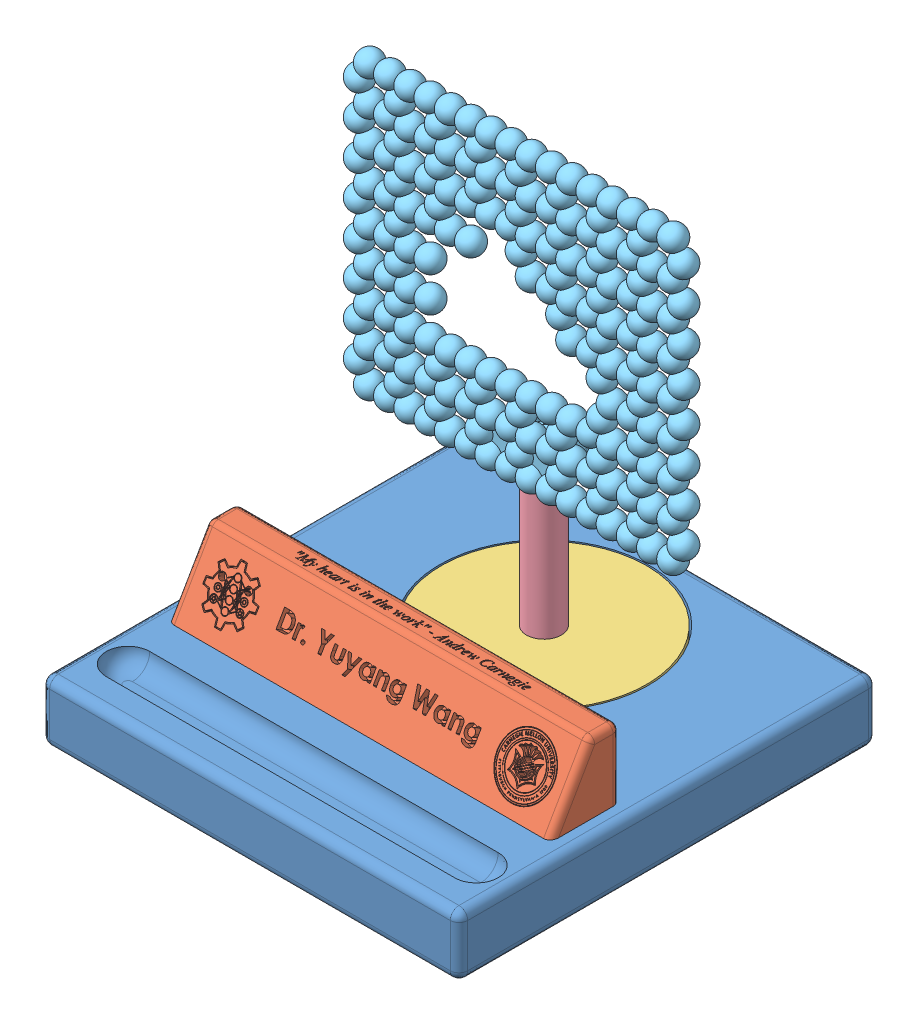
SolidWorks assembly PenHolderV1, configuration Default. Lengths in mm.
Overall size (152.4 180.63 152.4).
5 component instances, 5 part files, 7 mates.
Components (placement in the parent):
- Base-1: Base [9246K573] at origin size (152.4 22.23 152.4)
- NamePlate-1: NamePlate [Default] at (0 11.1125 23.8125) size (139.7 25.4 25.4)
- Mount-1: Mount [Default] at (0 -1.5875 -30.9563) size (74.93 12.7 74.93)
- Stand-1: Stand [Default] at (0 11.1125 -30.9563) size (12.7 50.8 12.7)
- Lattice-1: Lattice [Default] at (51.6359 70.0011 -22.7945) x (-0.999999 0 0.00103) z (-0.00103 0 -0.999999) size (126.32 110.13 23.32)
Mates (geometry in assembly coordinates):
- Coincident3: coincident anti-aligned: plane of Base-1 through (-76.2 11.1125 76.2) normal (0 1 0); plane of NamePlate-1 through (0 11.1125 23.8125) normal (0 -1 0)
- Distance11: distance = 12.7 mm: line of NamePlate-1 through (-67.31 11.1125 36.5125) axis (1 0 0); line of Base-1 through (63.5 11.1125 49.2125) axis (-1 0 0)
- Concentric2: concentric anti-aligned: circle of Base-1; circle of Mount-1
- Concentric3: concentric aligned: circle of Mount-1; circle of Stand-1
- Concentric4: concentric aligned: circle of Stand-1; circle of Lattice-1
- Coincident4: coincident anti-aligned: plane of Stand-1 through (0 61.9125 -30.9563) normal (0 1 0); plane of Lattice-1 through (11.0865 61.9125 -41.8027) normal (0 -1 0)
- Coincident5: coincident aligned: plane of Mount-1 through (0 11.1125 -30.9563) normal (0 1 0); circle of Stand-1
